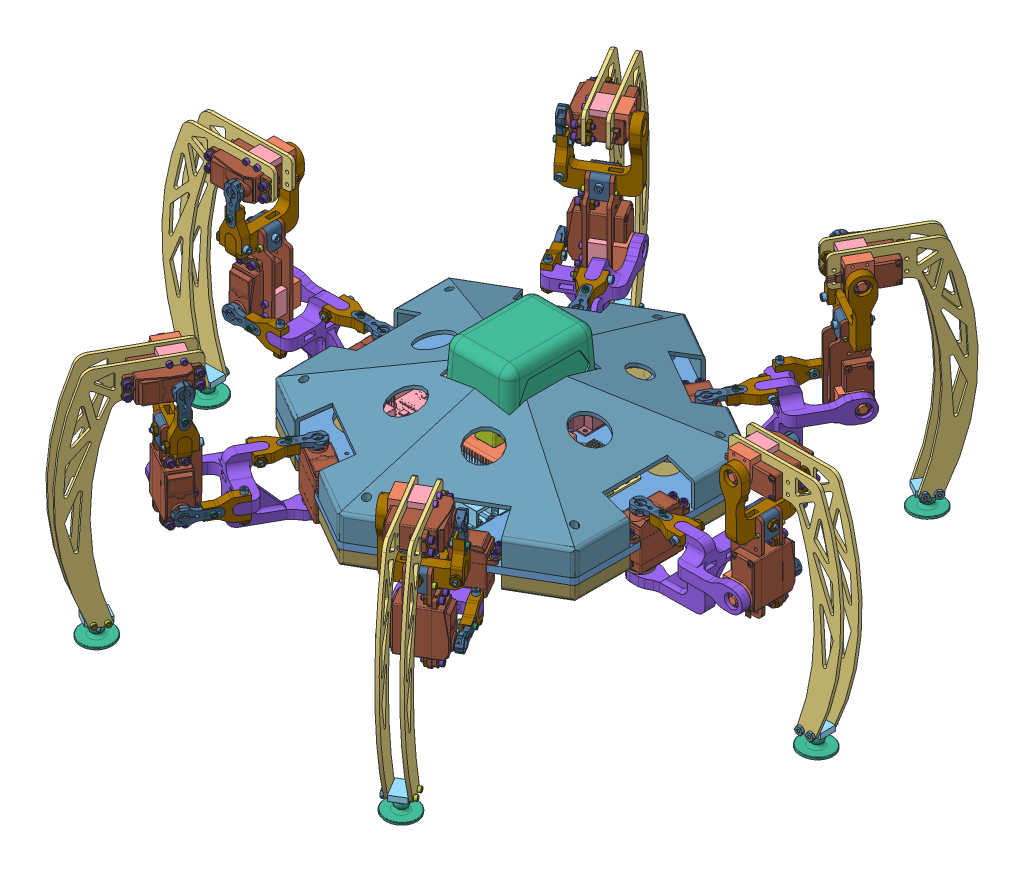
SolidWorks assembly Hexapod_(Hexagonal), configuration Défaut. Lengths in mm. (continued)
Components (placement in the parent): (continued)
- Foot+Tibia+Femur-8: Foot+Tibia+Femur [Défaut] at (76.9411 -25 93.0658) x (-0.5 0 -0.866025) z (0.866025 0 -0.5) size (210.19 223.27 63.83) (flexible) (continued)
  - Foot_(Long)-4: Foot_(Long) [Défaut] at (-141.7664 117.7478 -37.8795) x (0.999923 0.001668 -0.012321) z (0.012321 0 0.999924) size (104.1 223.13 60.64) (flexible) (continued)
    - HX-SHCS 0.138-32x0.5x0.5-N-17: HX-SHCS 0.138-32x0.5x0.5-N [HX-SHCS 0.138-32x0.5x0.5-N] at (44.9 15.2 35.772) x (0 0 -1) z (0.866025 0.5 0) size (16.21 5.74 5.74)
    - Narrow FW 0.138-2: Narrow FW 0.138 [Narrow FW 0.138] at (44.9 5.2 31.2) x (0 0 -1) z (-0.829316 0.55878 0) size (0.81 7.92 7.92)
    - Narrow FW 0.138-3: Narrow FW 0.138 [Narrow FW 0.138] at (-4.7 15.2 31.2) x (0 0 -1) z (-0.829316 0.55878 0) size (0.81 7.92 7.92)
    - Narrow FW 0.138-4: Narrow FW 0.138 [Narrow FW 0.138] at (44.9 15.2 31.2) x (0 0 -1) z (-0.829316 0.55878 0) size (0.81 7.92 7.92)
  - Tibia-3: Tibia [Défaut] at (-122.5709 19.4647 -38.1161) x (-0.006318 -0.99998 0.000078) z (0.012321 0 0.999924) size (129.02 61.26 61.64) (flexible)
    - Joint_(Tibia_to_foot)-1: Joint_(Tibia_to_foot) [Défaut] at (-62.6 10.2 -10) size (64 20 58.8)
    - DS3225MG-2: DS3225MG [Default] at (-10.1 10.2 45.8) x (-1 0 0) z (0 0 1) size (57.25 20.4 45.91)
    - Link-3: Link [Default] at (-10.1 22.9 11.1) x (0 -1 0) z (0 0 1) size (5 20.2 13.9)
    - Horn-2: Horn [Défaut] at (-10.1 10.2 48.8) x (-0.006319 0.99998 0) z (0 0 1) size (35.39 15.87 6)
    - Horn_attachment-2: Horn_attachment [Défaut] at (-10.2769 38.1994 44.8) x (0.006319 -0.99998 0) z (0 0 1) size (33 20 8)
    - Joint_attachment_(Tibia)-1: Joint_attachment_(Tibia) [Défaut] at (-62.6 10.2 25) size (19 20.4 13.9)
    - Tibia-1: Tibia [Défaut] at (-62.6 10.2 28) size (80 28 3)
    - Tibia-2: Tibia [Défaut] at (-62.6 10.2 11.1) size (80 28 3)
    - Bearing_mount_(Foot)-2: Bearing_mount_(Foot) [Default] at (-10.1 22.9 8.1) x (0 1 0) z (0 0 -1) size (25.3 20.2 17.1)
    - Bearing-2: Bearing [Default] at (-10.1 10.2 -6.7498) x (-0.993915 0.110147 0) z (0.110147 0.993915 0) size (13.87 4.75 13.87)
    - HX-SHCS 0.112-40x0.4375x0.4375-N-1: HX-SHCS 0.112-40x0.4375x0.4375-N [HX-SHCS 0.112-40x0.4375x0.4375-N] at (-10.2264 30.1996 51.6448) x (0 0 -1) z (-0.862849 -0.505462 0) size (13.96 4.65 4.65)
    - MSHXNUT 0.112-40-D-N-1: MSHXNUT 0.112-40-D-N [MSHXNUT 0.112-40-D-N] at (-10.2264 30.1996 40.8) x (-0.006319 0.99998 0) z (0 0 1) size (6.35 7.33 2.49)
    - HX-SHCS 0.112-40x1x0.75-N-1: HX-SHCS 0.112-40x1x0.75-N [HX-SHCS 0.112-40x1x0.75-N] at (-15.1 22.9 30.8448) x (0 0 -1) z (0 1 0) size (28.24 4.65 4.65)
    - HX-SHCS 0.112-40x1x0.75-N-2: HX-SHCS 0.112-40x1x0.75-N [HX-SHCS 0.112-40x1x0.75-N] at (-5.1 22.9 30.8448) x (0 0 -1) z (0 1 0) size (28.24 4.65 4.65)
    - HX-SHCS 0.138-32x0.5x0.5-N-1: HX-SHCS 0.138-32x0.5x0.5-N [HX-SHCS 0.138-32x0.5x0.5-N] at (-44.9 5.2 35.772) x (0 0 -1) z (0.866025 0.5 0) size (16.21 5.74 5.74)
    - Narrow FW 0.138-1: Narrow FW 0.138 [Narrow FW 0.138] at (-44.9 5.2 31.2) x (0 0 -1) z (-0.54947 -0.835514 0) size (0.81 7.92 7.92)
    - MSHXNUT 0.138-32-D-N-1: MSHXNUT 0.138-32-D-N [MSHXNUT 0.138-32-D-N] at (-44.9 5.2 25) x (0.866025 0.5 0) z (0 0 1) size (7.92 9.15 2.9)
    - MSHXNUT 0.138-32-D-N-2: MSHXNUT 0.138-32-D-N [MSHXNUT 0.138-32-D-N] at (4.7 5.2 25) x (0.866025 0.5 0) z (0 0 1) size (7.92 9.15 2.9)
    - MSHXNUT 0.138-32-D-N-3: MSHXNUT 0.138-32-D-N [MSHXNUT 0.138-32-D-N] at (-44.9 15.2 25) x (0.866025 0.5 0) z (0 0 1) size (7.92 9.15 2.9)
    - MSHXNUT 0.138-32-D-N-4: MSHXNUT 0.138-32-D-N [MSHXNUT 0.138-32-D-N] at (4.7 15.2 25) x (0.866025 0.5 0) z (0 0 1) size (7.92 9.15 2.9)
    - Narrow FW 0.138-2: Narrow FW 0.138 [Narrow FW 0.138] at (4.7 5.2 31.2) x (0 0 -1) z (-0.54947 -0.835514 0) size (0.81 7.92 7.92)
    - Narrow FW 0.138-3: Narrow FW 0.138 [Narrow FW 0.138] at (-44.9 15.2 31.2) x (0 0 -1) z (-0.54947 -0.835514 0) size (0.81 7.92 7.92)
    - Narrow FW 0.138-4: Narrow FW 0.138 [Narrow FW 0.138] at (4.7 15.2 31.2) x (0 0 -1) z (-0.54947 -0.835514 0) size (0.81 7.92 7.92)
    - HX-SHCS 0.138-32x0.5x0.5-N-2: HX-SHCS 0.138-32x0.5x0.5-N [HX-SHCS 0.138-32x0.5x0.5-N] at (4.7 5.2 35.772) x (0 0 -1) z (0.866025 0.5 0) size (16.21 5.74 5.74)
    - HX-SHCS 0.138-32x0.5x0.5-N-3: HX-SHCS 0.138-32x0.5x0.5-N [HX-SHCS 0.138-32x0.5x0.5-N] at (-44.9 15.2 35.772) x (0 0 -1) z (0.866025 0.5 0) size (16.21 5.74 5.74)
    - HX-SHCS 0.138-32x0.5x0.5-N-4: HX-SHCS 0.138-32x0.5x0.5-N [HX-SHCS 0.138-32x0.5x0.5-N] at (4.7 15.2 35.772) x (0 0 -1) z (0.866025 0.5 0) size (16.21 5.74 5.74)
    - HX-SHCS 0.112-40x0.875x0.875-N-1: HX-SHCS 0.112-40x0.875x0.875-N [HX-SHCS 0.112-40x0.875x0.875-N] at (-57.6 17.8 30.8448) x (0 0 -1) z (0 1 0) size (25.07 4.65 4.65)
    - HX-SHCS 0.112-40x0.875x0.875-N-2: HX-SHCS 0.112-40x0.875x0.875-N [HX-SHCS 0.112-40x0.875x0.875-N] at (-57.6 2.6 30.8448) x (0 0 -1) z (0 1 0) size (25.07 4.65 4.65)
    - HX-SHCS 0.138-32x1x1-N-1: HX-SHCS 0.138-32x1x1-N [HX-SHCS 0.138-32x1x1-N] at (-62.6 23.9052 18.05) x (0 -1 0) z (1 0 0) size (28.91 5.74 5.74)
    - MSHXNUT 0.138-32-D-N-5: MSHXNUT 0.138-32-D-N [MSHXNUT 0.138-32-D-N] at (-62.6 -2.8956 18.05) x (1 0 0) z (0 -1 0) size (7.92 9.15 2.9)
  - HX-SHCS 0.138-32x1x1-N-1: HX-SHCS 0.138-32x1x1-N [HX-SHCS 0.138-32x1x1-N] at (-69.7593 43.0052 6.0366) x (0 -1 0) z (-0.87212 0 -0.489292) size (28.91 5.74 5.74)
  - MSHXNUT 0.138-32-D-N-1: MSHXNUT 0.138-32-D-N [MSHXNUT 0.138-32-D-N] at (-69.7593 16.6044 6.0366) x (-0.87212 0 -0.489292) z (0 -1 0) size (7.92 9.15 2.9)
  - MSHXNUT 0.138-32-D-N-2: MSHXNUT 0.138-32-D-N [MSHXNUT 0.138-32-D-N] at (-124.2935 86.0804 6.7086) x (-0.000689 0.866008 -0.500029) z (-0.999904 0.006319 0.012321) size (7.92 9.15 2.9)
  - HX-SHCS 0.138-32x1x1-N-2: HX-SHCS 0.138-32x1x1-N [HX-SHCS 0.138-32x1x1-N] at (-97.8952 85.9135 6.3833) x (-0.999904 0.006319 0.012321) z (-0.012321 0 -0.999924) size (28.91 5.74 5.74)
- Foot+Tibia+Femur-9: Foot+Tibia+Femur [Défaut] at (119.0679 -25 -20.1) x (-1 0 0) z (0 0 -1) size (210.19 223.27 63.83) (flexible)
  - Femur-1: Femur [Défaut] at origin size (137.43 61.64 61.08) (flexible)
    - Joint_(Femur_to_tibia)-1: Joint_(Femur_to_tibia) [Défaut] at (-66.4348 29.5 -48.8085) x (0.999924 0 -0.012321) z (0.012321 0 0.999924) size (122 58.8 58.8)
    - Horn_attachment-3: Horn_attachment [Défaut] at (-38.1979 44.8 -29.755) x (0.999924 0 -0.012321) z (0 1 0) size (33 20 8)
    - Horn-3: Horn [Défaut] at (-10.2 48.8 -30.1) x (-0.999924 0 0.012321) z (0 1 0) size (35.39 15.87 6)
    - DS3225MG-3: DS3225MG [Default] at (-10.2 45.8 -30.1) x (0 0 1) z (0 1 0) size (57.25 20.4 45.91)
    - Bearing_mount_(Femur)-1: Bearing_mount_(Femur) [Default] at (2.5 22 -30.1) x (1 0 0) z (0 -1 0) size (35.3 20.2 31)
    - Bearing-3: Bearing [Default] at (-10.2 -6.7498 -30.1) x (0.400474 0 0.916308) z (-0.916308 0 0.400474) size (13.87 4.75 13.87)
    - MSHXNUT 0.112-40-D-N-1: MSHXNUT 0.112-40-D-N [MSHXNUT 0.112-40-D-N] at (-30.1985 40.8 -29.8536) x (-0.510633 0 -0.859799) z (0 1 0) size (6.35 7.33 2.49)
    - HX-SHCS 0.112-40x0.4375x0.4375-N-1: HX-SHCS 0.112-40x0.4375x0.4375-N [HX-SHCS 0.112-40x0.4375x0.4375-N] at (-30.1985 51.6448 -29.8536) x (0 -1 0) z (-0.489292 0 0.87212) size (13.96 4.65 4.65)
    - Narrow FW 0.138-1: Narrow FW 0.138 [Narrow FW 0.138] at (-15.2 31.2 4.7) x (0 -1 0) z (-0.829316 0 -0.55878) size (0.81 7.92 7.92)
    - HX-SHCS 0.138-32x0.5x0.5-N-1: HX-SHCS 0.138-32x0.5x0.5-N [HX-SHCS 0.138-32x0.5x0.5-N] at (-15.2 35.772 4.7) x (0 -1 0) z (0.866025 0 -0.5) size (16.21 5.74 5.74)
    - Narrow FW 0.138-2: Narrow FW 0.138 [Narrow FW 0.138] at (-15.2 31.2 -44.9) x (0 -1 0) z (-0.829316 0 -0.55878) size (0.81 7.92 7.92)
    - Narrow FW 0.138-3: Narrow FW 0.138 [Narrow FW 0.138] at (-5.2 31.2 4.7) x (0 -1 0) z (-0.829316 0 -0.55878) size (0.81 7.92 7.92)
    - Narrow FW 0.138-4: Narrow FW 0.138 [Narrow FW 0.138] at (-5.2 31.2 -44.9) x (0 -1 0) z (-0.829316 0 -0.55878) size (0.81 7.92 7.92)
    - HX-SHCS 0.138-32x0.5x0.5-N-2: HX-SHCS 0.138-32x0.5x0.5-N [HX-SHCS 0.138-32x0.5x0.5-N] at (-15.2 35.772 -44.9) x (0 -1 0) z (0.866025 0 -0.5) size (16.21 5.74 5.74)
    - HX-SHCS 0.138-32x0.5x0.5-N-3: HX-SHCS 0.138-32x0.5x0.5-N [HX-SHCS 0.138-32x0.5x0.5-N] at (-5.2 35.772 4.7) x (0 -1 0) z (0.866025 0 -0.5) size (16.21 5.74 5.74)
    - HX-SHCS 0.138-32x0.5x0.5-N-4: HX-SHCS 0.138-32x0.5x0.5-N [HX-SHCS 0.138-32x0.5x0.5-N] at (-5.2 35.772 -44.9) x (0 -1 0) z (0.866025 0 -0.5) size (16.21 5.74 5.74)
    - MSHXNUT 0.138-32-D-N-1: MSHXNUT 0.138-32-D-N [MSHXNUT 0.138-32-D-N] at (-52.0379 44.8 -16.6879) x (-0.86596 -0.5 0.010671) z (0.012321 0 0.999924) size (7.92 9.15 2.9)
    - HX-SHCS 0.138-32x1x1-N-2: HX-SHCS 0.138-32x1x1-N [HX-SHCS 0.138-32x1x1-N] at (-52.3632 44.8 -43.0867) x (0.012321 0 0.999924) z (-0.86596 -0.5 0.010671) size (28.91 5.74 5.74)
  - Foot_(Long)-4: Foot_(Long) [Défaut] at (-141.7664 117.7478 -37.8795) x (0.999923 0.001668 -0.012321) z (0.012321 0 0.999924) size (104.1 223.13 60.64) (flexible)
    - DS3225MG-1: DS3225MG [Default] at (30.1 10.2 45.8) x (-1 0 0) z (0 0 1) size (57.25 20.4 45.91)
    - Bearing-1: Bearing [Default] at (30.1 10.2 -6.7498) x (-0.568255 0.822853 0) z (0.822853 0.568255 0) size (13.87 4.75 13.87)
    - Bearing_mount_(Foot)-1: Bearing_mount_(Foot) [Default] at (30.1 22.9 8.1) x (0 1 0) z (0 0 -1) size (25.3 20.2 17.1)
    - Foot_(Long)-1: Foot_(Long) [Default] at (18.7 14 25) size (103.08 208 3)
    - Link-1: Link [Default] at (30.1 22.9 11.1) x (0 -1 0) z (0 0 1) size (5 20.2 13.9)
    - Foot_(Long)-2: Foot_(Long) [Default] at (18.7 14 8.1) size (103.08 208 3)
    - Joint_(Foot_to_slipper)-2: Joint_(Foot_to_slipper) [Default] at (-21.9427 -177.5 11.1) x (0 1 0) z (0 0 1) size (15 20.2 13.9)
    - Horn-1: Horn [Défaut] at (30.1 10.2 48.8) x (-0.007987 -0.999968 0) z (0 0 1) size (35.39 15.87 6)
    - Horn_attachment-1: Horn_attachment [Défaut] at (29.8764 -17.7991 44.8) x (0.007987 0.999968 0) z (0 0 1) size (33 20 8)
    - Slipper-1: Slipper [Défaut] at (-21.7184 -191.9896 17.7406) x (0.999392 0.031392 0.015197) z (-0.013787 -0.044657 0.998907) size (30 10.55 30)
    - HX-SHCS 0.112-40x0.4375x0.4375-N-15: HX-SHCS 0.112-40x0.4375x0.4375-N [HX-SHCS 0.112-40x0.4375x0.4375-N] at (29.9403 -9.7994 51.6448) x (0 0 -1) z (0.869991 0.493067 0) size (13.96 4.65 4.65)
    - MSHXNUT 0.112-40-D-N-7: MSHXNUT 0.112-40-D-N [MSHXNUT 0.112-40-D-N] at (29.9403 -9.7994 40.8) x (-0.007987 -0.999968 0) z (0 0 1) size (6.35 7.33 2.49)
    - HX-SHCS 0.112-40x0.875x0.875-N-9: HX-SHCS 0.112-40x0.875x0.875-N [HX-SHCS 0.112-40x0.875x0.875-N] at (-26.9427 -177.5 30.8448) x (0 0 -1) z (0 1 0) size (25.07 4.65 4.65)
    - MSHXNUT 0.112-40-D-N-4: MSHXNUT 0.112-40-D-N [MSHXNUT 0.112-40-D-N] at (-26.9427 -177.5 8.1) x (0.866025 -0.5 0) z (0 0 1) size (6.35 7.33 2.49)
    - HX-SHCS 0.112-40x0.875x0.875-N-11: HX-SHCS 0.112-40x0.875x0.875-N [HX-SHCS 0.112-40x0.875x0.875-N] at (-16.9427 -177.5 30.8448) x (0 0 -1) z (0 1 0) size (25.07 4.65 4.65)
    - MSHXNUT 0.112-40-D-N-6: MSHXNUT 0.112-40-D-N [MSHXNUT 0.112-40-D-N] at (-16.9427 -177.5 8.1) x (0.866025 -0.5 0) z (0 0 1) size (6.35 7.33 2.49)
    - HX-SHCS 0.112-40x1x0.75-N-13: HX-SHCS 0.112-40x1x0.75-N [HX-SHCS 0.112-40x1x0.75-N] at (25.1 22.9 30.8448) x (0 0 -1) z (0 1 0) size (28.24 4.65 4.65)
    - HX-SHCS 0.112-40x1x0.75-N-14: HX-SHCS 0.112-40x1x0.75-N [HX-SHCS 0.112-40x1x0.75-N] at (35.1 22.9 30.8448) x (0 0 -1) z (0 1 0) size (28.24 4.65 4.65)
    - HX-SHCS 0.138-32x0.5x0.5-N-14: HX-SHCS 0.138-32x0.5x0.5-N [HX-SHCS 0.138-32x0.5x0.5-N] at (-4.7 5.2 35.772) x (0 0 -1) z (0.866025 0.5 0) size (16.21 5.74 5.74)
    - Narrow FW 0.138-1: Narrow FW 0.138 [Narrow FW 0.138] at (-4.7 5.2 31.2) x (0 0 -1) z (-0.829316 0.55878 0) size (0.81 7.92 7.92)
    - MSHXNUT 0.138-32-D-N-1: MSHXNUT 0.138-32-D-N [MSHXNUT 0.138-32-D-N] at (-4.7 5.2 25) x (0.866025 0.5 0) z (0 0 1) size (7.92 9.15 2.9)
    - MSHXNUT 0.138-32-D-N-2: MSHXNUT 0.138-32-D-N [MSHXNUT 0.138-32-D-N] at (44.9 5.2 25) x (0.866025 0.5 0) z (0 0 1) size (7.92 9.15 2.9)
    - MSHXNUT 0.138-32-D-N-3: MSHXNUT 0.138-32-D-N [MSHXNUT 0.138-32-D-N] at (-4.7 15.2 25) x (0.866025 0.5 0) z (0 0 1) size (7.92 9.15 2.9)
    - MSHXNUT 0.138-32-D-N-4: MSHXNUT 0.138-32-D-N [MSHXNUT 0.138-32-D-N] at (44.9 15.2 25) x (0.866025 0.5 0) z (0 0 1) size (7.92 9.15 2.9)
    - HX-SHCS 0.138-32x0.5x0.5-N-15: HX-SHCS 0.138-32x0.5x0.5-N [HX-SHCS 0.138-32x0.5x0.5-N] at (44.9 5.2 35.772) x (0 0 -1) z (0.866025 0.5 0) size (16.21 5.74 5.74)
    - HX-SHCS 0.138-32x0.5x0.5-N-16: HX-SHCS 0.138-32x0.5x0.5-N [HX-SHCS 0.138-32x0.5x0.5-N] at (-4.7 15.2 35.772) x (0 0 -1) z (0.866025 0.5 0) size (16.21 5.74 5.74)
    - HX-SHCS 0.138-32x0.5x0.5-N-17: HX-SHCS 0.138-32x0.5x0.5-N [HX-SHCS 0.138-32x0.5x0.5-N] at (44.9 15.2 35.772) x (0 0 -1) z (0.866025 0.5 0) size (16.21 5.74 5.74)
    - Narrow FW 0.138-2: Narrow FW 0.138 [Narrow FW 0.138] at (44.9 5.2 31.2) x (0 0 -1) z (-0.829316 0.55878 0) size (0.81 7.92 7.92)
    - Narrow FW 0.138-3: Narrow FW 0.138 [Narrow FW 0.138] at (-4.7 15.2 31.2) x (0 0 -1) z (-0.829316 0.55878 0) size (0.81 7.92 7.92)
    - Narrow FW 0.138-4: Narrow FW 0.138 [Narrow FW 0.138] at (44.9 15.2 31.2) x (0 0 -1) z (-0.829316 0.55878 0) size (0.81 7.92 7.92)
  - Tibia-3: Tibia [Défaut] at (-122.5709 19.4647 -38.1161) x (-0.006318 -0.99998 0.000078) z (0.012321 0 0.999924) size (129.02 61.26 61.64) (flexible)
    - Joint_(Tibia_to_foot)-1: Joint_(Tibia_to_foot) [Défaut] at (-62.6 10.2 -10) size (64 20 58.8)
    - DS3225MG-2: DS3225MG [Default] at (-10.1 10.2 45.8) x (-1 0 0) z (0 0 1) size (57.25 20.4 45.91)
    - Link-3: Link [Default] at (-10.1 22.9 11.1) x (0 -1 0) z (0 0 1) size (5 20.2 13.9)
    - Horn-2: Horn [Défaut] at (-10.1 10.2 48.8) x (-0.006319 0.99998 0) z (0 0 1) size (35.39 15.87 6)
    - Horn_attachment-2: Horn_attachment [Défaut] at (-10.2769 38.1994 44.8) x (0.006319 -0.99998 0) z (0 0 1) size (33 20 8)
    - Joint_attachment_(Tibia)-1: Joint_attachment_(Tibia) [Défaut] at (-62.6 10.2 25) size (19 20.4 13.9)
    - Tibia-1: Tibia [Défaut] at (-62.6 10.2 28) size (80 28 3)
    - Tibia-2: Tibia [Défaut] at (-62.6 10.2 11.1) size (80 28 3)
    - Bearing_mount_(Foot)-2: Bearing_mount_(Foot) [Default] at (-10.1 22.9 8.1) x (0 1 0) z (0 0 -1) size (25.3 20.2 17.1)
    - Bearing-2: Bearing [Default] at (-10.1 10.2 -6.7498) x (-0.993915 0.110147 0) z (0.110147 0.993915 0) size (13.87 4.75 13.87)
    - HX-SHCS 0.112-40x0.4375x0.4375-N-1: HX-SHCS 0.112-40x0.4375x0.4375-N [HX-SHCS 0.112-40x0.4375x0.4375-N] at (-10.2264 30.1996 51.6448) x (0 0 -1) z (-0.862849 -0.505462 0) size (13.96 4.65 4.65)
    - MSHXNUT 0.112-40-D-N-1: MSHXNUT 0.112-40-D-N [MSHXNUT 0.112-40-D-N] at (-10.2264 30.1996 40.8) x (-0.006319 0.99998 0) z (0 0 1) size (6.35 7.33 2.49)
    - HX-SHCS 0.112-40x1x0.75-N-1: HX-SHCS 0.112-40x1x0.75-N [HX-SHCS 0.112-40x1x0.75-N] at (-15.1 22.9 30.8448) x (0 0 -1) z (0 1 0) size (28.24 4.65 4.65)
    - HX-SHCS 0.112-40x1x0.75-N-2: HX-SHCS 0.112-40x1x0.75-N [HX-SHCS 0.112-40x1x0.75-N] at (-5.1 22.9 30.8448) x (0 0 -1) z (0 1 0) size (28.24 4.65 4.65)
    - HX-SHCS 0.138-32x0.5x0.5-N-1: HX-SHCS 0.138-32x0.5x0.5-N [HX-SHCS 0.138-32x0.5x0.5-N] at (-44.9 5.2 35.772) x (0 0 -1) z (0.866025 0.5 0) size (16.21 5.74 5.74)
    - Narrow FW 0.138-1: Narrow FW 0.138 [Narrow FW 0.138] at (-44.9 5.2 31.2) x (0 0 -1) z (-0.54947 -0.835514 0) size (0.81 7.92 7.92)
    - MSHXNUT 0.138-32-D-N-1: MSHXNUT 0.138-32-D-N [MSHXNUT 0.138-32-D-N] at (-44.9 5.2 25) x (0.866025 0.5 0) z (0 0 1) size (7.92 9.15 2.9)
    - MSHXNUT 0.138-32-D-N-2: MSHXNUT 0.138-32-D-N [MSHXNUT 0.138-32-D-N] at (4.7 5.2 25) x (0.866025 0.5 0) z (0 0 1) size (7.92 9.15 2.9)
    - MSHXNUT 0.138-32-D-N-3: MSHXNUT 0.138-32-D-N [MSHXNUT 0.138-32-D-N] at (-44.9 15.2 25) x (0.866025 0.5 0) z (0 0 1) size (7.92 9.15 2.9)
    - MSHXNUT 0.138-32-D-N-4: MSHXNUT 0.138-32-D-N [MSHXNUT 0.138-32-D-N] at (4.7 15.2 25) x (0.866025 0.5 0) z (0 0 1) size (7.92 9.15 2.9)
    - Narrow FW 0.138-2: Narrow FW 0.138 [Narrow FW 0.138] at (4.7 5.2 31.2) x (0 0 -1) z (-0.54947 -0.835514 0) size (0.81 7.92 7.92)
    - Narrow FW 0.138-3: Narrow FW 0.138 [Narrow FW 0.138] at (-44.9 15.2 31.2) x (0 0 -1) z (-0.54947 -0.835514 0) size (0.81 7.92 7.92)
    - Narrow FW 0.138-4: Narrow FW 0.138 [Narrow FW 0.138] at (4.7 15.2 31.2) x (0 0 -1) z (-0.54947 -0.835514 0) size (0.81 7.92 7.92)
    - HX-SHCS 0.138-32x0.5x0.5-N-2: HX-SHCS 0.138-32x0.5x0.5-N [HX-SHCS 0.138-32x0.5x0.5-N] at (4.7 5.2 35.772) x (0 0 -1) z (0.866025 0.5 0) size (16.21 5.74 5.74)
    - HX-SHCS 0.138-32x0.5x0.5-N-3: HX-SHCS 0.138-32x0.5x0.5-N [HX-SHCS 0.138-32x0.5x0.5-N] at (-44.9 15.2 35.772) x (0 0 -1) z (0.866025 0.5 0) size (16.21 5.74 5.74)
    - HX-SHCS 0.138-32x0.5x0.5-N-4: HX-SHCS 0.138-32x0.5x0.5-N [HX-SHCS 0.138-32x0.5x0.5-N] at (4.7 15.2 35.772) x (0 0 -1) z (0.866025 0.5 0) size (16.21 5.74 5.74)
    - HX-SHCS 0.112-40x0.875x0.875-N-1: HX-SHCS 0.112-40x0.875x0.875-N [HX-SHCS 0.112-40x0.875x0.875-N] at (-57.6 17.8 30.8448) x (0 0 -1) z (0 1 0) size (25.07 4.65 4.65)
    - HX-SHCS 0.112-40x0.875x0.875-N-2: HX-SHCS 0.112-40x0.875x0.875-N [HX-SHCS 0.112-40x0.875x0.875-N] at (-57.6 2.6 30.8448) x (0 0 -1) z (0 1 0) size (25.07 4.65 4.65)
    - HX-SHCS 0.138-32x1x1-N-1: HX-SHCS 0.138-32x1x1-N [HX-SHCS 0.138-32x1x1-N] at (-62.6 23.9052 18.05) x (0 -1 0) z (1 0 0) size (28.91 5.74 5.74)
    - MSHXNUT 0.138-32-D-N-5: MSHXNUT 0.138-32-D-N [MSHXNUT 0.138-32-D-N] at (-62.6 -2.8956 18.05) x (1 0 0) z (0 -1 0) size (7.92 9.15 2.9)
  - HX-SHCS 0.138-32x1x1-N-1: HX-SHCS 0.138-32x1x1-N [HX-SHCS 0.138-32x1x1-N] at (-69.7593 43.0052 6.0366) x (0 -1 0) z (-0.87212 0 -0.489292) size (28.91 5.74 5.74)
  - MSHXNUT 0.138-32-D-N-1: MSHXNUT 0.138-32-D-N [MSHXNUT 0.138-32-D-N] at (-69.7593 16.6044 6.0366) x (-0.87212 0 -0.489292) z (0 -1 0) size (7.92 9.15 2.9)
  - MSHXNUT 0.138-32-D-N-2: MSHXNUT 0.138-32-D-N [MSHXNUT 0.138-32-D-N] at (-124.2935 86.0804 6.7086) x (-0.000689 0.866008 -0.500029) z (-0.999904 0.006319 0.012321) size (7.92 9.15 2.9)
  - HX-SHCS 0.138-32x1x1-N-2: HX-SHCS 0.138-32x1x1-N [HX-SHCS 0.138-32x1x1-N] at (-97.8952 85.9135 6.3833) x (-0.999904 0.006319 0.012321) z (-0.012321 0 -0.999924) size (28.91 5.74 5.74)
- Foot+Tibia+Femur-10: Foot+Tibia+Femur [Défaut] at (42.1268 -25 -113.1658) x (-0.5 0 0.866025) z (-0.866025 0 -0.5) size (210.19 223.27 63.83) (flexible)
  - Femur-1: Femur [Défaut] at origin size (137.43 61.64 61.08) (flexible)
    - Joint_(Femur_to_tibia)-1: Joint_(Femur_to_tibia) [Défaut] at (-66.4348 29.5 -48.8085) x (0.999924 0 -0.012321) z (0.012321 0 0.999924) size (122 58.8 58.8)
    - Horn_attachment-3: Horn_attachment [Défaut] at (-38.1979 44.8 -29.755) x (0.999924 0 -0.012321) z (0 1 0) size (33 20 8)
    - Horn-3: Horn [Défaut] at (-10.2 48.8 -30.1) x (-0.999924 0 0.012321) z (0 1 0) size (35.39 15.87 6)
    - DS3225MG-3: DS3225MG [Default] at (-10.2 45.8 -30.1) x (0 0 1) z (0 1 0) size (57.25 20.4 45.91)
    - Bearing_mount_(Femur)-1: Bearing_mount_(Femur) [Default] at (2.5 22 -30.1) x (1 0 0) z (0 -1 0) size (35.3 20.2 31)
    - Bearing-3: Bearing [Default] at (-10.2 -6.7498 -30.1) x (0.400474 0 0.916308) z (-0.916308 0 0.400474) size (13.87 4.75 13.87)
    - MSHXNUT 0.112-40-D-N-1: MSHXNUT 0.112-40-D-N [MSHXNUT 0.112-40-D-N] at (-30.1985 40.8 -29.8536) x (-0.510633 0 -0.859799) z (0 1 0) size (6.35 7.33 2.49)
    - HX-SHCS 0.112-40x0.4375x0.4375-N-1: HX-SHCS 0.112-40x0.4375x0.4375-N [HX-SHCS 0.112-40x0.4375x0.4375-N] at (-30.1985 51.6448 -29.8536) x (0 -1 0) z (-0.489292 0 0.87212) size (13.96 4.65 4.65)
    - Narrow FW 0.138-1: Narrow FW 0.138 [Narrow FW 0.138] at (-15.2 31.2 4.7) x (0 -1 0) z (-0.829316 0 -0.55878) size (0.81 7.92 7.92)
    - HX-SHCS 0.138-32x0.5x0.5-N-1: HX-SHCS 0.138-32x0.5x0.5-N [HX-SHCS 0.138-32x0.5x0.5-N] at (-15.2 35.772 4.7) x (0 -1 0) z (0.866025 0 -0.5) size (16.21 5.74 5.74)
    - Narrow FW 0.138-2: Narrow FW 0.138 [Narrow FW 0.138] at (-15.2 31.2 -44.9) x (0 -1 0) z (-0.829316 0 -0.55878) size (0.81 7.92 7.92)
    - Narrow FW 0.138-3: Narrow FW 0.138 [Narrow FW 0.138] at (-5.2 31.2 4.7) x (0 -1 0) z (-0.829316 0 -0.55878) size (0.81 7.92 7.92)
    - Narrow FW 0.138-4: Narrow FW 0.138 [Narrow FW 0.138] at (-5.2 31.2 -44.9) x (0 -1 0) z (-0.829316 0 -0.55878) size (0.81 7.92 7.92)
    - HX-SHCS 0.138-32x0.5x0.5-N-2: HX-SHCS 0.138-32x0.5x0.5-N [HX-SHCS 0.138-32x0.5x0.5-N] at (-15.2 35.772 -44.9) x (0 -1 0) z (0.866025 0 -0.5) size (16.21 5.74 5.74)
    - HX-SHCS 0.138-32x0.5x0.5-N-3: HX-SHCS 0.138-32x0.5x0.5-N [HX-SHCS 0.138-32x0.5x0.5-N] at (-5.2 35.772 4.7) x (0 -1 0) z (0.866025 0 -0.5) size (16.21 5.74 5.74)
    - HX-SHCS 0.138-32x0.5x0.5-N-4: HX-SHCS 0.138-32x0.5x0.5-N [HX-SHCS 0.138-32x0.5x0.5-N] at (-5.2 35.772 -44.9) x (0 -1 0) z (0.866025 0 -0.5) size (16.21 5.74 5.74)
    - MSHXNUT 0.138-32-D-N-1: MSHXNUT 0.138-32-D-N [MSHXNUT 0.138-32-D-N] at (-52.0379 44.8 -16.6879) x (-0.86596 -0.5 0.010671) z (0.012321 0 0.999924) size (7.92 9.15 2.9)
    - HX-SHCS 0.138-32x1x1-N-2: HX-SHCS 0.138-32x1x1-N [HX-SHCS 0.138-32x1x1-N] at (-52.3632 44.8 -43.0867) x (0.012321 0 0.999924) z (-0.86596 -0.5 0.010671) size (28.91 5.74 5.74)
  - Foot_(Long)-4: Foot_(Long) [Défaut] at (-141.7664 117.7478 -37.8795) x (0.999923 0.001668 -0.012321) z (0.012321 0 0.999924) size (104.1 223.13 60.64) (flexible)
    - DS3225MG-1: DS3225MG [Default] at (30.1 10.2 45.8) x (-1 0 0) z (0 0 1) size (57.25 20.4 45.91)
    - Bearing-1: Bearing [Default] at (30.1 10.2 -6.7498) x (-0.568255 0.822853 0) z (0.822853 0.568255 0) size (13.87 4.75 13.87)
    - Bearing_mount_(Foot)-1: Bearing_mount_(Foot) [Default] at (30.1 22.9 8.1) x (0 1 0) z (0 0 -1) size (25.3 20.2 17.1)
    - Foot_(Long)-1: Foot_(Long) [Default] at (18.7 14 25) size (103.08 208 3)
    - Link-1: Link [Default] at (30.1 22.9 11.1) x (0 -1 0) z (0 0 1) size (5 20.2 13.9)
    - Foot_(Long)-2: Foot_(Long) [Default] at (18.7 14 8.1) size (103.08 208 3)
    - Joint_(Foot_to_slipper)-2: Joint_(Foot_to_slipper) [Default] at (-21.9427 -177.5 11.1) x (0 1 0) z (0 0 1) size (15 20.2 13.9)
    - Horn-1: Horn [Défaut] at (30.1 10.2 48.8) x (-0.007987 -0.999968 0) z (0 0 1) size (35.39 15.87 6)
    - Horn_attachment-1: Horn_attachment [Défaut] at (29.8764 -17.7991 44.8) x (0.007987 0.999968 0) z (0 0 1) size (33 20 8)
    - Slipper-1: Slipper [Défaut] at (-21.7184 -191.9896 17.7406) x (0.999392 0.031392 0.015197) z (-0.013787 -0.044657 0.998907) size (30 10.55 30)
    - HX-SHCS 0.112-40x0.4375x0.4375-N-15: HX-SHCS 0.112-40x0.4375x0.4375-N [HX-SHCS 0.112-40x0.4375x0.4375-N] at (29.9403 -9.7994 51.6448) x (0 0 -1) z (0.869991 0.493067 0) size (13.96 4.65 4.65)
    - MSHXNUT 0.112-40-D-N-7: MSHXNUT 0.112-40-D-N [MSHXNUT 0.112-40-D-N] at (29.9403 -9.7994 40.8) x (-0.007987 -0.999968 0) z (0 0 1) size (6.35 7.33 2.49)
    - HX-SHCS 0.112-40x0.875x0.875-N-9: HX-SHCS 0.112-40x0.875x0.875-N [HX-SHCS 0.112-40x0.875x0.875-N] at (-26.9427 -177.5 30.8448) x (0 0 -1) z (0 1 0) size (25.07 4.65 4.65)
    - MSHXNUT 0.112-40-D-N-4: MSHXNUT 0.112-40-D-N [MSHXNUT 0.112-40-D-N] at (-26.9427 -177.5 8.1) x (0.866025 -0.5 0) z (0 0 1) size (6.35 7.33 2.49)
    - HX-SHCS 0.112-40x0.875x0.875-N-11: HX-SHCS 0.112-40x0.875x0.875-N [HX-SHCS 0.112-40x0.875x0.875-N] at (-16.9427 -177.5 30.8448) x (0 0 -1) z (0 1 0) size (25.07 4.65 4.65)
    - MSHXNUT 0.112-40-D-N-6: MSHXNUT 0.112-40-D-N [MSHXNUT 0.112-40-D-N] at (-16.9427 -177.5 8.1) x (0.866025 -0.5 0) z (0 0 1) size (6.35 7.33 2.49)
    - HX-SHCS 0.112-40x1x0.75-N-13: HX-SHCS 0.112-40x1x0.75-N [HX-SHCS 0.112-40x1x0.75-N] at (25.1 22.9 30.8448) x (0 0 -1) z (0 1 0) size (28.24 4.65 4.65)
    - HX-SHCS 0.112-40x1x0.75-N-14: HX-SHCS 0.112-40x1x0.75-N [HX-SHCS 0.112-40x1x0.75-N] at (35.1 22.9 30.8448) x (0 0 -1) z (0 1 0) size (28.24 4.65 4.65)
    - HX-SHCS 0.138-32x0.5x0.5-N-14: HX-SHCS 0.138-32x0.5x0.5-N [HX-SHCS 0.138-32x0.5x0.5-N] at (-4.7 5.2 35.772) x (0 0 -1) z (0.866025 0.5 0) size (16.21 5.74 5.74)
    - Narrow FW 0.138-1: Narrow FW 0.138 [Narrow FW 0.138] at (-4.7 5.2 31.2) x (0 0 -1) z (-0.829316 0.55878 0) size (0.81 7.92 7.92)
    - MSHXNUT 0.138-32-D-N-1: MSHXNUT 0.138-32-D-N [MSHXNUT 0.138-32-D-N] at (-4.7 5.2 25) x (0.866025 0.5 0) z (0 0 1) size (7.92 9.15 2.9)
    - MSHXNUT 0.138-32-D-N-2: MSHXNUT 0.138-32-D-N [MSHXNUT 0.138-32-D-N] at (44.9 5.2 25) x (0.866025 0.5 0) z (0 0 1) size (7.92 9.15 2.9)
    - MSHXNUT 0.138-32-D-N-3: MSHXNUT 0.138-32-D-N [MSHXNUT 0.138-32-D-N] at (-4.7 15.2 25) x (0.866025 0.5 0) z (0 0 1) size (7.92 9.15 2.9)
    - MSHXNUT 0.138-32-D-N-4: MSHXNUT 0.138-32-D-N [MSHXNUT 0.138-32-D-N] at (44.9 15.2 25) x (0.866025 0.5 0) z (0 0 1) size (7.92 9.15 2.9)
    - HX-SHCS 0.138-32x0.5x0.5-N-15: HX-SHCS 0.138-32x0.5x0.5-N [HX-SHCS 0.138-32x0.5x0.5-N] at (44.9 5.2 35.772) x (0 0 -1) z (0.866025 0.5 0) size (16.21 5.74 5.74)
    - HX-SHCS 0.138-32x0.5x0.5-N-16: HX-SHCS 0.138-32x0.5x0.5-N [HX-SHCS 0.138-32x0.5x0.5-N] at (-4.7 15.2 35.772) x (0 0 -1) z (0.866025 0.5 0) size (16.21 5.74 5.74)
    - HX-SHCS 0.138-32x0.5x0.5-N-17: HX-SHCS 0.138-32x0.5x0.5-N [HX-SHCS 0.138-32x0.5x0.5-N] at (44.9 15.2 35.772) x (0 0 -1) z (0.866025 0.5 0) size (16.21 5.74 5.74)
    - Narrow FW 0.138-2: Narrow FW 0.138 [Narrow FW 0.138] at (44.9 5.2 31.2) x (0 0 -1) z (-0.829316 0.55878 0) size (0.81 7.92 7.92)
    - Narrow FW 0.138-3: Narrow FW 0.138 [Narrow FW 0.138] at (-4.7 15.2 31.2) x (0 0 -1) z (-0.829316 0.55878 0) size (0.81 7.92 7.92)
    - Narrow FW 0.138-4: Narrow FW 0.138 [Narrow FW 0.138] at (44.9 15.2 31.2) x (0 0 -1) z (-0.829316 0.55878 0) size (0.81 7.92 7.92)
  - Tibia-3: Tibia [Défaut] at (-122.5709 19.4647 -38.1161) x (-0.006318 -0.99998 0.000078) z (0.012321 0 0.999924) size (129.02 61.26 61.64) (flexible)
    - Joint_(Tibia_to_foot)-1: Joint_(Tibia_to_foot) [Défaut] at (-62.6 10.2 -10) size (64 20 58.8)
    - DS3225MG-2: DS3225MG [Default] at (-10.1 10.2 45.8) x (-1 0 0) z (0 0 1) size (57.25 20.4 45.91)
    - Link-3: Link [Default] at (-10.1 22.9 11.1) x (0 -1 0) z (0 0 1) size (5 20.2 13.9)
    - Horn-2: Horn [Défaut] at (-10.1 10.2 48.8) x (-0.006319 0.99998 0) z (0 0 1) size (35.39 15.87 6)
    - Horn_attachment-2: Horn_attachment [Défaut] at (-10.2769 38.1994 44.8) x (0.006319 -0.99998 0) z (0 0 1) size (33 20 8)
    - Joint_attachment_(Tibia)-1: Joint_attachment_(Tibia) [Défaut] at (-62.6 10.2 25) size (19 20.4 13.9)
    - Tibia-1: Tibia [Défaut] at (-62.6 10.2 28) size (80 28 3)
    - Tibia-2: Tibia [Défaut] at (-62.6 10.2 11.1) size (80 28 3)
    - Bearing_mount_(Foot)-2: Bearing_mount_(Foot) [Default] at (-10.1 22.9 8.1) x (0 1 0) z (0 0 -1) size (25.3 20.2 17.1)
    - Bearing-2: Bearing [Default] at (-10.1 10.2 -6.7498) x (-0.993915 0.110147 0) z (0.110147 0.993915 0) size (13.87 4.75 13.87)
    - HX-SHCS 0.112-40x0.4375x0.4375-N-1: HX-SHCS 0.112-40x0.4375x0.4375-N [HX-SHCS 0.112-40x0.4375x0.4375-N] at (-10.2264 30.1996 51.6448) x (0 0 -1) z (-0.862849 -0.505462 0) size (13.96 4.65 4.65)
    - MSHXNUT 0.112-40-D-N-1: MSHXNUT 0.112-40-D-N [MSHXNUT 0.112-40-D-N] at (-10.2264 30.1996 40.8) x (-0.006319 0.99998 0) z (0 0 1) size (6.35 7.33 2.49)
    - HX-SHCS 0.112-40x1x0.75-N-1: HX-SHCS 0.112-40x1x0.75-N [HX-SHCS 0.112-40x1x0.75-N] at (-15.1 22.9 30.8448) x (0 0 -1) z (0 1 0) size (28.24 4.65 4.65)
    - HX-SHCS 0.112-40x1x0.75-N-2: HX-SHCS 0.112-40x1x0.75-N [HX-SHCS 0.112-40x1x0.75-N] at (-5.1 22.9 30.8448) x (0 0 -1) z (0 1 0) size (28.24 4.65 4.65)
    - HX-SHCS 0.138-32x0.5x0.5-N-1: HX-SHCS 0.138-32x0.5x0.5-N [HX-SHCS 0.138-32x0.5x0.5-N] at (-44.9 5.2 35.772) x (0 0 -1) z (0.866025 0.5 0) size (16.21 5.74 5.74)
    - Narrow FW 0.138-1: Narrow FW 0.138 [Narrow FW 0.138] at (-44.9 5.2 31.2) x (0 0 -1) z (-0.54947 -0.835514 0) size (0.81 7.92 7.92)
    - MSHXNUT 0.138-32-D-N-1: MSHXNUT 0.138-32-D-N [MSHXNUT 0.138-32-D-N] at (-44.9 5.2 25) x (0.866025 0.5 0) z (0 0 1) size (7.92 9.15 2.9)
    - MSHXNUT 0.138-32-D-N-2: MSHXNUT 0.138-32-D-N [MSHXNUT 0.138-32-D-N] at (4.7 5.2 25) x (0.866025 0.5 0) z (0 0 1) size (7.92 9.15 2.9)
    - MSHXNUT 0.138-32-D-N-3: MSHXNUT 0.138-32-D-N [MSHXNUT 0.138-32-D-N] at (-44.9 15.2 25) x (0.866025 0.5 0) z (0 0 1) size (7.92 9.15 2.9)
    - MSHXNUT 0.138-32-D-N-4: MSHXNUT 0.138-32-D-N [MSHXNUT 0.138-32-D-N] at (4.7 15.2 25) x (0.866025 0.5 0) z (0 0 1) size (7.92 9.15 2.9)
    - Narrow FW 0.138-2: Narrow FW 0.138 [Narrow FW 0.138] at (4.7 5.2 31.2) x (0 0 -1) z (-0.54947 -0.835514 0) size (0.81 7.92 7.92)
    - Narrow FW 0.138-3: Narrow FW 0.138 [Narrow FW 0.138] at (-44.9 15.2 31.2) x (0 0 -1) z (-0.54947 -0.835514 0) size (0.81 7.92 7.92)
    - Narrow FW 0.138-4: Narrow FW 0.138 [Narrow FW 0.138] at (4.7 15.2 31.2) x (0 0 -1) z (-0.54947 -0.835514 0) size (0.81 7.92 7.92)
    - HX-SHCS 0.138-32x0.5x0.5-N-2: HX-SHCS 0.138-32x0.5x0.5-N [HX-SHCS 0.138-32x0.5x0.5-N] at (4.7 5.2 35.772) x (0 0 -1) z (0.866025 0.5 0) size (16.21 5.74 5.74)
    - HX-SHCS 0.138-32x0.5x0.5-N-3: HX-SHCS 0.138-32x0.5x0.5-N [HX-SHCS 0.138-32x0.5x0.5-N] at (-44.9 15.2 35.772) x (0 0 -1) z (0.866025 0.5 0) size (16.21 5.74 5.74)
    - HX-SHCS 0.138-32x0.5x0.5-N-4: HX-SHCS 0.138-32x0.5x0.5-N [HX-SHCS 0.138-32x0.5x0.5-N] at (4.7 15.2 35.772) x (0 0 -1) z (0.866025 0.5 0) size (16.21 5.74 5.74)
    - HX-SHCS 0.112-40x0.875x0.875-N-1: HX-SHCS 0.112-40x0.875x0.875-N [HX-SHCS 0.112-40x0.875x0.875-N] at (-57.6 17.8 30.8448) x (0 0 -1) z (0 1 0) size (25.07 4.65 4.65)
    - HX-SHCS 0.112-40x0.875x0.875-N-2: HX-SHCS 0.112-40x0.875x0.875-N [HX-SHCS 0.112-40x0.875x0.875-N] at (-57.6 2.6 30.8448) x (0 0 -1) z (0 1 0) size (25.07 4.65 4.65)
    - HX-SHCS 0.138-32x1x1-N-1: HX-SHCS 0.138-32x1x1-N [HX-SHCS 0.138-32x1x1-N] at (-62.6 23.9052 18.05) x (0 -1 0) z (1 0 0) size (28.91 5.74 5.74)
    - MSHXNUT 0.138-32-D-N-5: MSHXNUT 0.138-32-D-N [MSHXNUT 0.138-32-D-N] at (-62.6 -2.8956 18.05) x (1 0 0) z (0 -1 0) size (7.92 9.15 2.9)
  - HX-SHCS 0.138-32x1x1-N-1: HX-SHCS 0.138-32x1x1-N [HX-SHCS 0.138-32x1x1-N] at (-69.7593 43.0052 6.0366) x (0 -1 0) z (-0.87212 0 -0.489292) size (28.91 5.74 5.74)
  - MSHXNUT 0.138-32-D-N-1: MSHXNUT 0.138-32-D-N [MSHXNUT 0.138-32-D-N] at (-69.7593 16.6044 6.0366) x (-0.87212 0 -0.489292) z (0 -1 0) size (7.92 9.15 2.9)
  - MSHXNUT 0.138-32-D-N-2: MSHXNUT 0.138-32-D-N [MSHXNUT 0.138-32-D-N] at (-124.2935 86.0804 6.7086) x (-0.000689 0.866008 -0.500029) z (-0.999904 0.006319 0.012321) size (7.92 9.15 2.9)
  - HX-SHCS 0.138-32x1x1-N-2: HX-SHCS 0.138-32x1x1-N [HX-SHCS 0.138-32x1x1-N] at (-97.8952 85.9135 6.3833) x (-0.999904 0.006319 0.012321) z (-0.012321 0 -0.999924) size (28.91 5.74 5.74)
